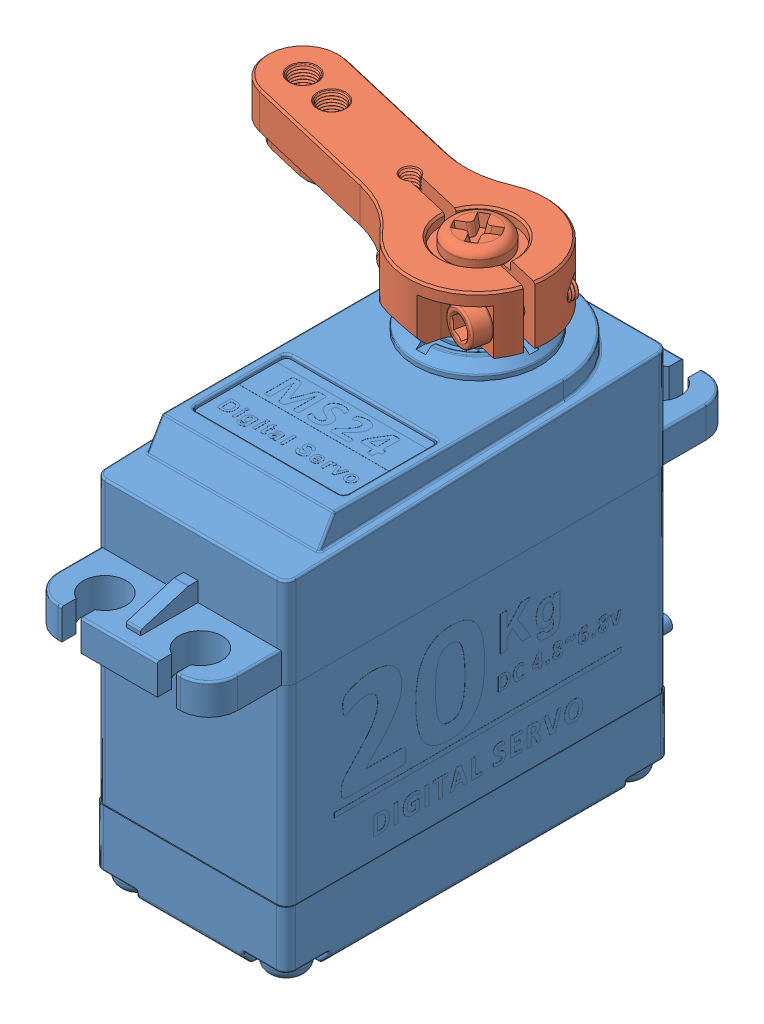
SolidWorks assembly servo, configuration Default. Lengths in mm.
Overall size (39.26 49.37 55.6).
2 component instances, 2 part files, 2 mates.
Components (placement in the parent):
- DS3218MG MS24 Digital Servo 270^servo-1: DS3218MG MS24 Digital Servo 270^servo [Default] at origin size (20.1 45.99 55.6) (virtual)
- Servo Arm^servo-1: Servo Arm^servo [Default] x (0.228641 0 -0.973511) z (0.973511 0 0.228641) size (14.5 6.95 35.53) (virtual)
Mates (geometry in assembly coordinates):
- Concentric1: concentric anti-aligned: cylinder of Servo Arm^DS3240 Digital Servo-1 through (0 18.4 0) axis (0 -1 0) radius 2.5; cylinder of DS3218MG MS24 Digital Servo 270-1 through (0 13.5 0) axis (0 1 0) radius 3.8
- Coincident1: coincident anti-aligned: plane of Copy of DS3218MG MS24 Digital Servo 270^DS3240 Digital Servo-1 through (0 18.4 0) normal (0 1 0); plane of Servo Arm^DS3240 Digital Servo-1 through (0 18.4 0) normal (0 -1 0)
